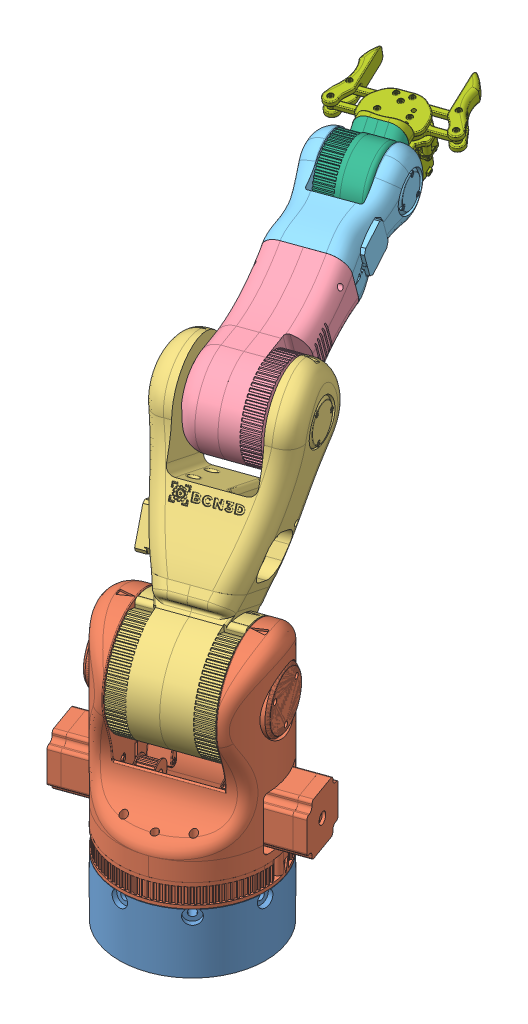
SolidWorks assembly Desktop_Arm_URDF_Assembly, configuration Default. Lengths in mm.
Overall size (380.37 632.42 627.96).
7 component instances, 7 part files, 13 mates.
Components (placement in the parent):
- desktop_arm_base-1: desktop_arm_base [Default] at (32.0572 72.0407 -86.3519) size (160 65.48 160)
- desktop_arm_link_1-1: desktop_arm_link_1 [Default] at (-125.7179 71.0407 -28.0138) x (0.759411 0 -0.650612) z (0.650612 0 0.759411) size (227.97 229.44 160)
- desktop_arm_link_2-1: desktop_arm_link_2 [Default] at (-140.5744 148.7231 -70.3536) x (0.765122 0.108729 -0.634639) z (0.635665 -0.284544 0.71761) size (193.51 273.26 276.23)
- desktop_arm_link_3-1: desktop_arm_link_3 [Default] at (-107.0459 108.7873 25.5967) x (0.759411 0 -0.650612) z (0.650612 0 0.759411) size (129.57 129.76 191.35)
- desktop_arm_link_4-1: desktop_arm_link_4 [Default] at (92.9986 772.9797 221.5952) x (-0.994179 0.106047 0.019025) z (-0.056607 -0.664378 0.74525) size (118.48 111.83 147.54)
- desktop_arm_link_5-1: desktop_arm_link_5 [Default] at (-45.5411 984.1067 -165.0501) x (-0.970037 -0.228787 0.081759) z (0.014143 0.282773 0.959083) size (67.24 81.08 90.31)
- desktop_arm_gripper-1: desktop_arm_gripper [Default] at (-171.2796 132.6372 -312.1766) x (0.841349 0.31015 -0.44265) z (0.53096 -0.627412 0.569593) size (119.91 84.94 107.98)
Mates (geometry in assembly coordinates):
- Concentric1: concentric anti-aligned: cylinder of desktop_arm_base-1 through (32.0498 88.1844 156.1481) axis (0 1 0) radius 4; cylinder of desktop_arm_link_1-1 through (32.0498 108.2844 156.1481) axis (0 -1 0) radius 4
- Coincident1: coincident anti-aligned: plane of desktop_arm_base-1 through (32.0498 88.1844 156.1481) normal (0 1 0); plane of desktop_arm_link_1-1 through (32.0498 88.1844 156.1481) normal (0 -1 0)
- Concentric2: concentric aligned: cylinder of desktop_arm_link_1-1 through (97.963 253.6844 132.5802) axis (-0.941618 0 0.336684) radius 4; cylinder of desktop_arm_link_2-1 through (77.0271 253.6844 140.0661) axis (-0.941618 0 0.336684) radius 4.15
- Distance1: distance = 1.016 mm anti-aligned: plane of desktop_arm_link_2-1 through (-12.4266 253.6844 172.0511) normal (-0.941618 0 0.336684); plane of desktop_arm_link_1-1 through (18.6018 133.6844 261.8468) normal (0.941618 0 -0.336684)
- Concentric3: concentric anti-aligned: cylinder of desktop_arm_link_2-1 through (-60.0785 454.4898 90.7587) axis (0.941618 0 -0.336684) radius 4.15; cylinder of desktop_arm_link_3-1 through (35.9815 454.4898 56.4115) axis (-0.941618 0 0.336684) radius 4.15
- Distance2: distance = 1.016 mm anti-aligned: plane of desktop_arm_link_3-1 through (-79.4298 466.8859 -42.118) normal (-0.941618 0 0.336684); plane of desktop_arm_link_2-1 through (15.3753 367.9122 226.0446) normal (0.941618 0 -0.336684)
- Concentric4: concentric aligned: cylinder of desktop_arm_link_3-1 through (-36.5668 497.1422 -37.3345) axis (0.314887 -0.353962 0.880657) radius 4; cylinder of desktop_arm_link_4-1 through (-40.3455 501.3898 -47.9024) axis (0.314887 -0.353962 0.880657) radius 4.15
- Coincident4: coincident anti-aligned: plane of desktop_arm_link_3-1 through (-34.5338 499.62 -45.0142) normal (-0.314887 0.353962 -0.880657); plane of desktop_arm_link_4-1 through (9.3274 546.6165 -41.8079) normal (0.314887 -0.353962 0.880657)
- Concentric5: concentric aligned: cylinder of desktop_arm_link_4-1 through (-26.2834 533.4807 -142.2286) axis (-0.942266 -0.005207 0.334824) radius 4.15; cylinder of desktop_arm_link_5-1 through (-46.0559 533.3714 -135.2027) axis (-0.942266 -0.005207 0.334824) radius 4.1
- Distance3: distance = 1.016 mm anti-aligned: plane of desktop_arm_link_5-1 through (-91.2847 533.1215 -119.1311) normal (-0.942266 -0.005207 0.334824); plane of desktop_arm_link_4-1 through (-56.6312 546.2521 -18.3702) normal (0.942266 0.005207 -0.334824)
- Concentric6: concentric anti-aligned: cylinder of desktop_arm_link_5-1 through (-87.5483 553.2573 -144.1429) axis (-0.328544 0.207721 -0.921364) radius 1.65; cylinder of desktop_arm_gripper-1 through (-95.1048 558.0349 -165.3343) axis (0.328544 -0.207721 0.921364) radius 1.6
- Concentric7: concentric anti-aligned: cylinder of desktop_arm_link_5-1 through (-64.9339 553.3823 -152.1787) axis (-0.328544 0.207721 -0.921364) radius 1.65; cylinder of desktop_arm_gripper-1 through (-72.4904 558.1599 -173.37) axis (0.328544 -0.207721 0.921364) radius 1.6
- Coincident6: coincident anti-aligned: plane of desktop_arm_link_5-1 through (-59.5262 541.888 -172.9786) normal (-0.328544 0.207721 -0.921364); plane of desktop_arm_gripper-1 through (-62.4427 497.8302 -181.8714) normal (0.328544 -0.207721 0.921364)
